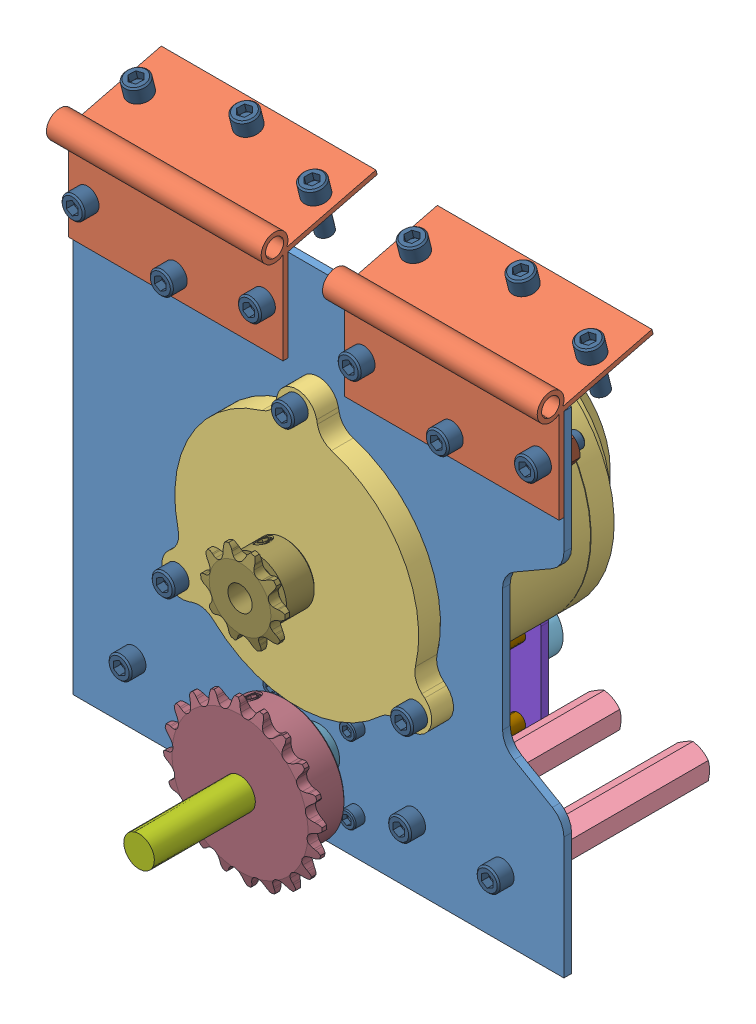
SolidWorks assembly Subassem - Steering Motor, configuration Default. Lengths in mm.
Overall size (203.2 231.02 172.82).
54 component instances, 14 part files, 101 mates.
Components (placement in the parent):
- Motor Mount-1: Motor Mount [Default] at origin size (203.2 203.2 3.17)
- Hinges-1: Hinges [Default] at (0 105.8998 5.5035) size (203.2 49.24 48.03)
- Motor-1: Motor [Default] at (0 0 -78.6404) x (1 0 0) z (0 -1 0) size (111.79 120.23 113.74)
- Standoff 3in 0.25-20-1: Standoff 3in 0.25-20 [92230A345] at (76.2 -76.2 -41.275) size (12.7 14.66 77.95)
- Standoff 3in 0.25-20-2: Standoff 3in 0.25-20 [92230A345] at (39.5531 -76.2 -41.275) size (12.7 14.66 77.95)
- Standoff 3in 0.25-20-3: Standoff 3in 0.25-20 [92230A345] at (-39.5531 -76.2 -41.275) size (12.7 14.66 77.95)
- Standoff 3in 0.25-20-4: Standoff 3in 0.25-20 [92230A345] at (-76.2 -76.2 -41.275) size (12.7 14.66 77.95)
- Potentiometer-1: Potentiometer [Default] at (0 -69.8325 -90.17) x (1 0 0) z (0 -1 0) size (22.23 39.37 22.23)
- Shaft Coupler 0.25-0.50-1: Shaft Coupler 0.25-0.50 [3084K31] at (0 -69.8325 -39.6875) x (0 0 -1) z (-0.419694 0.907666 0) size (47.67 31.75 31.75)
- Shaft 0.5in-1: Shaft 0.5in [Default] at (0 -69.85 17.145) x (-0.735553 0.677467 0) z (0 0 1) size (12.7 12.7 114.3)
- Pot Plate-2: Pot Plate [Default] at (0 -69.8325 -68.2625) size (50.8 50.8 3.17)
- Standoff 3in 8-32-1: Standoff 3in 8-32 [Default] at (-15.875 -53.9575 -34.925) size (6.35 6.35 63.5)
- Standoff 3in 8-32-7: Standoff 3in 8-32 [Default] at (15.875 -85.7075 -34.925) size (6.35 6.35 63.5)
- Standoff 3in 8-32-8: Standoff 3in 8-32 [Default] at (15.875 -53.9575 -34.925) size (6.35 6.35 63.5)
- Standoff 3in 8-32-9: Standoff 3in 8-32 [Default] at (-15.875 -85.7425 -34.925) size (6.35 6.35 63.5)
- Socket Head Cap Screw_AI-1: Socket Head Cap Screw_AI [HX-SHCS 0.25-28x0.625x0.625-N] at (-76.2 -76.2 6.35) x (0 0 -1) z (1 0 0) size (22.23 9.53 9.53)
- Socket Head Cap Screw_AI-2: Socket Head Cap Screw_AI [HX-SHCS 0.25-28x0.625x0.625-N] at (-39.5531 -76.2 6.35) x (0 0 -1) z (1 0 0) size (22.23 9.53 9.53)
- Socket Head Cap Screw_AI-3: Socket Head Cap Screw_AI [HX-SHCS 0.25-28x0.625x0.625-N] at (39.5531 -76.2 6.35) x (0 0 -1) z (1 0 0) size (22.23 9.53 9.53)
- Socket Head Cap Screw_AI-4: Socket Head Cap Screw_AI [HX-SHCS 0.25-28x0.625x0.625-N] at (76.2 -76.2 6.35) x (0 0 -1) z (1 0 0) size (22.23 9.53 9.53)
- Socket Head Cap Screw_AI-6: Socket Head Cap Screw_AI [HX-SHCS 0.25-28x0.625x0.625-N] at (-93.6625 80.9625 8.3344) x (0 0 -1) z (1 0 0) size (22.23 9.53 9.53)
- Socket Head Cap Screw_AI-7: Socket Head Cap Screw_AI [HX-SHCS 0.25-28x0.625x0.625-N] at (-57.15 72.2313 8.3344) x (0 0 -1) z (1 0 0) size (22.23 9.53 9.53)
- Socket Head Cap Screw_AI-8: Socket Head Cap Screw_AI [HX-SHCS 0.25-28x0.625x0.625-N] at (-20.6375 80.9625 8.3344) x (0 0 -1) z (1 0 0) size (22.23 9.53 9.53)
- Socket Head Cap Screw_AI-9: Socket Head Cap Screw_AI [HX-SHCS 0.25-28x0.625x0.625-N] at (20.6375 80.9625 8.3344) x (0 0 -1) z (1 0 0) size (22.23 9.53 9.53)
- Socket Head Cap Screw_AI-10: Socket Head Cap Screw_AI [HX-SHCS 0.25-28x0.625x0.625-N] at (57.15 72.2313 8.3344) x (0 0 -1) z (1 0 0) size (22.23 9.53 9.53)
- Socket Head Cap Screw_AI-11: Socket Head Cap Screw_AI [HX-SHCS 0.25-28x0.625x0.625-N] at (93.6625 80.9625 8.3344) x (0 0 -1) z (1 0 0) size (22.23 9.53 9.53)
- Socket Head Cap Screw_AI-31: Socket Head Cap Screw_AI [HX-SHCS 0.25-20x1x1-N] at (0 57 15.35) x (0 0 -1) z (1 0 0) size (31.75 9.53 9.53)
- Socket Head Cap Screw_AI-32: Socket Head Cap Screw_AI [HX-SHCS 0.25-20x1x1-N] at (-49.3634 -28.5 15.35) x (0 0 -1) z (1 0 0) size (31.75 9.53 9.53)
- Socket Head Cap Screw_AI-33: Socket Head Cap Screw_AI [HX-SHCS 0.25-20x1x1-N] at (49.3634 -28.5 15.35) x (0 0 -1) z (1 0 0) size (31.75 9.53 9.53)
- Hex Nut_AI-2: Hex Nut_AI [HNUT 0.2500-28-D-N] at (-93.6625 80.9625 -3.175) size (11.11 12.83 5.74)
- Hex Nut_AI-3: Hex Nut_AI [HNUT 0.2500-28-D-N] at (-57.15 72.2313 -4.085) size (11.11 12.83 5.74)
- Hex Nut_AI-4: Hex Nut_AI [HNUT 0.2500-28-D-N] at (-20.6375 80.9625 -8.9154) x (0.923728 0.383049 0) z (0 0 -1) size (11.11 12.83 5.74)
- Hex Nut_AI-5: Hex Nut_AI [HNUT 0.2500-28-D-N] at (20.6375 80.9625 -8.9154) x (0.923728 0.383049 0) z (0 0 -1) size (11.11 12.83 5.74)
- Hex Nut_AI-6: Hex Nut_AI [HNUT 0.2500-28-D-N] at (57.15 72.2313 -8.9154) x (0.923728 0.383049 0) z (0 0 -1) size (11.11 12.83 5.74)
- Hex Nut_AI-7: Hex Nut_AI [HNUT 0.2500-28-D-N] at (93.6625 80.9625 -8.9154) x (0.923728 0.383049 0) z (0 0 -1) size (11.11 12.83 5.74)
- Hex Nut_AI-8: Hex Nut_AI [HNUT 0.2500-20-D-N] at (0 57 -8.9154) x (0.923728 0.383049 0) z (0 0 -1) size (11.11 12.83 5.74)
- Hex Nut_AI-9: Hex Nut_AI [HNUT 0.2500-20-D-N] at (-49.3634 -28.5 -8.9154) x (0.923728 0.383049 0) z (0 0 -1) size (11.11 12.83 5.74)
- Hex Nut_AI-10: Hex Nut_AI [HNUT 0.2500-20-D-N] at (49.3634 -28.5 -8.9154) x (0.923728 0.383049 0) z (0 0 -1) size (11.11 12.83 5.74)
- Socket Head Cap Screw_AI-35: Socket Head Cap Screw_AI [HX-SHCS 0.164-32x0.5x0.5-N] at (-15.875 -53.9575 4.1656) x (0 0 -1) z (1 0 0) size (16.87 6.86 6.86)
- Socket Head Cap Screw_AI-36: Socket Head Cap Screw_AI [HX-SHCS 0.164-32x0.5x0.5-N] at (-15.875 -85.7425 4.1656) x (0 0 -1) z (1 0 0) size (16.87 6.86 6.86)
- Socket Head Cap Screw_AI-37: Socket Head Cap Screw_AI [HX-SHCS 0.164-32x0.5x0.5-N] at (15.875 -53.9575 4.1656) x (0 0 -1) z (1 0 0) size (16.87 6.86 6.86)
- Socket Head Cap Screw_AI-38: Socket Head Cap Screw_AI [HX-SHCS 0.164-32x0.5x0.5-N] at (15.875 -85.7425 4.1656) x (0 0 -1) z (1 0 0) size (16.87 6.86 6.86)
- Socket Head Cap Screw_AI-39: Socket Head Cap Screw_AI [HX-SHCS 0.164-32x0.5x0.5-N] at (15.875 -53.9575 -74.0156) x (0 0 1) z (-1 0 0) size (16.87 6.86 6.86)
- Socket Head Cap Screw_AI-40: Socket Head Cap Screw_AI [HX-SHCS 0.164-32x0.5x0.5-N] at (15.875 -85.7075 -74.0156) x (0 0 1) z (-1 0 0) size (16.87 6.86 6.86)
- Socket Head Cap Screw_AI-41: Socket Head Cap Screw_AI [HX-SHCS 0.164-32x0.5x0.5-N] at (-15.875 -85.7075 -74.0156) x (0 0 1) z (-1 0 0) size (16.87 6.86 6.86)
- Socket Head Cap Screw_AI-42: Socket Head Cap Screw_AI [HX-SHCS 0.164-32x0.5x0.5-N] at (-15.875 -53.9575 -74.0156) x (0 0 1) z (-1 0 0) size (16.87 6.86 6.86)
- Socket Head Cap Screw_AI-44: Socket Head Cap Screw_AI [HX-SHCS 0.25-28x0.625x0.625-N] at (-93.6625 114.6795 -18.0082) x (0 -0.970296 -0.241922) z (0.241922 -0.234736 0.941474) size (22.23 9.53 9.53)
- Socket Head Cap Screw_AI-45: Socket Head Cap Screw_AI [HX-SHCS 0.25-28x0.625x0.625-N] at (-57.15 116.7918 -26.4801) x (0 -0.970296 -0.241922) z (0.241922 -0.234736 0.941474) size (22.23 9.53 9.53)
- Socket Head Cap Screw_AI-46: Socket Head Cap Screw_AI [HX-SHCS 0.25-28x0.625x0.625-N] at (-20.6375 114.6795 -18.0082) x (0 -0.970296 -0.241922) z (0.241922 -0.234736 0.941474) size (22.23 9.53 9.53)
- Socket Head Cap Screw_AI-47: Socket Head Cap Screw_AI [HX-SHCS 0.25-28x0.625x0.625-N] at (20.6375 114.6795 -18.0082) x (0 -0.970296 -0.241922) z (0.241922 -0.234736 0.941474) size (22.23 9.53 9.53)
- Socket Head Cap Screw_AI-48: Socket Head Cap Screw_AI [HX-SHCS 0.25-28x0.625x0.625-N] at (57.15 116.7918 -26.4801) x (0 -0.970296 -0.241922) z (0.241922 -0.234736 0.941474) size (22.23 9.53 9.53)
- Socket Head Cap Screw_AI-49: Socket Head Cap Screw_AI [HX-SHCS 0.25-28x0.625x0.625-N] at (93.6625 114.6795 -18.0082) x (0 -0.970296 -0.241922) z (0.241922 -0.234736 0.941474) size (22.23 9.53 9.53)
- Sprocket - 10 Tooth-1: Sprocket - 10 Tooth [6280K321] at (0 0 30.3614) x (-0.923728 -0.383049 0) z (0 0 -1) size (33.82 35.03 19.05)
- Sprocket - 15 Tooth-1: Sprocket - 15 Tooth [6280K384] at (0 -69.85 30.3614) x (-0.923728 -0.383049 0) z (0 0 -1) size (65.79 65.79 19.05)
- Roller Bearing 0.5in-1: Roller Bearing 0.5in [5905K23] at (0 -69.85 -2.3118) x (0.999532 0.030579 0) z (0 0 1) size (17.46 17.46 12.7)
Mates (geometry in assembly coordinates):
- Concentric1: concentric aligned: cylinder of Motor Mount-1 through (-93.6625 80.9625 0) axis (0 0 1) radius 3.2639; cylinder of Hinges-1 through (-93.6625 80.9625 0) axis (0 0 1) radius 4.3656
- Concentric2: concentric aligned: cylinder of Motor Mount-1 through (-57.15 72.2313 0) axis (0 0 1) radius 3.2639; cylinder of Hinges-1 through (-57.15 72.2313 0) axis (0 0 1) radius 4.3656
- Coincident1: coincident anti-aligned: plane of Motor Mount-1 through (0 0 0) normal (0 0 1); plane of Hinges-1 through (101.6 105.8998 0) normal (0 0 -1)
- Coincident2: coincident aligned: circle of Motor Mount-1; circle of Motor-1
- Concentric3: concentric anti-aligned: cylinder of Motor Mount-1 through (-49.3634 -28.5 -3.175) axis (0 0 1) radius 4.25; cylinder of Motor-1 through (-49.3634 -28.5 9) axis (0 0 -1) radius 4.25
- Concentric7: concentric anti-aligned: circle of Motor Mount-1; circle of Standoff 3in 0.25-20-1
- Coincident5: coincident anti-aligned: plane of Motor Mount-1 through (0 0 -3.175) normal (0 0 -1); plane of Standoff 3in 0.25-20-1 through (76.2 -68.8677 -3.175) normal (0 0 1)
- Coincident6: coincident anti-aligned: plane of Motor Mount-1 through (0 0 -3.175) normal (0 0 -1); plane of Standoff 3in 0.25-20-2 through (39.5531 -68.8677 -3.175) normal (0 0 1)
- Concentric8: concentric anti-aligned: circle of Motor Mount-1; circle of Standoff 3in 0.25-20-2
- Concentric9: concentric anti-aligned: circle of Motor Mount-1; circle of Standoff 3in 0.25-20-3
- Coincident7: coincident anti-aligned: plane of Motor Mount-1 through (0 0 -3.175) normal (0 0 -1); plane of Standoff 3in 0.25-20-3 through (-39.5531 -68.8677 -3.175) normal (0 0 1)
- Concentric10: concentric anti-aligned: circle of Motor Mount-1; circle of Standoff 3in 0.25-20-4
- Coincident8: coincident anti-aligned: plane of Motor Mount-1 through (0 0 -3.175) normal (0 0 -1); plane of Standoff 3in 0.25-20-4 through (-76.2 -68.8677 -3.175) normal (0 0 1)
- Concentric13: concentric aligned: cylinder of Motor Mount-1 through (-76.2 -76.2 0) axis (0 0 1) radius 3.2639; cylinder of Socket Head Cap Screw_AI-1 through (-76.2 -76.2 38.1) axis (0 0 1) radius 4.7625
- Coincident11: coincident anti-aligned: plane of Motor Mount-1 through (0 0 0) normal (0 0 1); plane of Socket Head Cap Screw_AI-1 through (-76.2 -71.4375 0) normal (0 0 -1)
- Concentric14: concentric aligned: cylinder of Motor Mount-1 through (-39.5531 -76.2 0) axis (0 0 1) radius 3.2639; cylinder of Socket Head Cap Screw_AI-2 through (-39.5531 -76.2 38.1) axis (0 0 1) radius 4.7625
- Coincident12: coincident anti-aligned: plane of Motor Mount-1 through (0 0 0) normal (0 0 1); plane of Socket Head Cap Screw_AI-2 through (-39.5531 -71.4375 0) normal (0 0 -1)
- Concentric15: concentric aligned: cylinder of Motor Mount-1 through (39.5531 -76.2 0) axis (0 0 1) radius 3.2639; cylinder of Socket Head Cap Screw_AI-3 through (39.5531 -76.2 38.1) axis (0 0 1) radius 4.7625
- Coincident13: coincident anti-aligned: plane of Motor Mount-1 through (0 0 0) normal (0 0 1); plane of Socket Head Cap Screw_AI-3 through (39.5531 -71.4375 0) normal (0 0 -1)
- Concentric16: concentric aligned: cylinder of Motor Mount-1 through (76.2 -76.2 0) axis (0 0 1) radius 3.2639; cylinder of Socket Head Cap Screw_AI-4 through (76.2 -76.2 38.1) axis (0 0 1) radius 4.7625
- Coincident14: coincident anti-aligned: plane of Motor Mount-1 through (0 0 0) normal (0 0 1); plane of Socket Head Cap Screw_AI-4 through (76.2 -71.4375 0) normal (0 0 -1)
- Concentric18: concentric aligned: cylinder of Hinges-1 through (-93.6625 80.9625 0) axis (0 0 1) radius 4.3656; cylinder of Socket Head Cap Screw_AI-6 through (-93.6625 80.9625 40.0844) axis (0 0 1) radius 4.7625
- Coincident16: coincident anti-aligned: plane of Hinges-1 through (101.6 105.8998 1.9844) normal (0 0 1); plane of Socket Head Cap Screw_AI-6 through (-93.6625 85.725 1.9844) normal (0 0 -1)
- Concentric19: concentric aligned: cylinder of Hinges-1 through (-57.15 72.2313 0) axis (0 0 1) radius 4.3656; cylinder of Socket Head Cap Screw_AI-7 through (-57.15 72.2313 40.0844) axis (0 0 1) radius 4.7625
- Coincident17: coincident anti-aligned: plane of Hinges-1 through (101.6 105.8998 1.9844) normal (0 0 1); plane of Socket Head Cap Screw_AI-7 through (-57.15 76.9938 1.9844) normal (0 0 -1)
- Concentric20: concentric aligned: cylinder of Hinges-1 through (-20.6375 80.9625 0) axis (0 0 1) radius 4.3656; cylinder of Socket Head Cap Screw_AI-8 through (-20.6375 80.9625 40.0844) axis (0 0 1) radius 4.7625
- Coincident18: coincident anti-aligned: plane of Hinges-1 through (101.6 105.8998 1.9844) normal (0 0 1); plane of Socket Head Cap Screw_AI-8 through (-20.6375 85.725 1.9844) normal (0 0 -1)
- Concentric21: concentric aligned: cylinder of Hinges-1 through (20.6375 80.9625 0) axis (0 0 1) radius 4.3656; cylinder of Socket Head Cap Screw_AI-9 through (20.6375 80.9625 40.0844) axis (0 0 1) radius 4.7625
- Coincident19: coincident anti-aligned: plane of Hinges-1 through (101.6 105.8998 1.9844) normal (0 0 1); plane of Socket Head Cap Screw_AI-9 through (20.6375 85.725 1.9844) normal (0 0 -1)
- Concentric22: concentric aligned: cylinder of Hinges-1 through (57.15 72.2313 0) axis (0 0 1) radius 4.3656; cylinder of Socket Head Cap Screw_AI-10 through (57.15 72.2313 40.0844) axis (0 0 1) radius 4.7625
- Coincident20: coincident anti-aligned: plane of Hinges-1 through (101.6 105.8998 1.9844) normal (0 0 1); plane of Socket Head Cap Screw_AI-10 through (57.15 76.9938 1.9844) normal (0 0 -1)
- Concentric23: concentric aligned: cylinder of Hinges-1 through (93.6625 80.9625 0) axis (0 0 1) radius 4.3656; cylinder of Socket Head Cap Screw_AI-11 through (93.6625 80.9625 40.0844) axis (0 0 1) radius 4.7625
- Coincident21: coincident anti-aligned: plane of Hinges-1 through (101.6 105.8998 1.9844) normal (0 0 1); plane of Socket Head Cap Screw_AI-11 through (93.6625 85.725 1.9844) normal (0 0 -1)
- Concentric32: concentric anti-aligned: cylinder of Potentiometer-1 through (0 -69.8325 -90.17) axis (0 0 -1) radius 3.175; cylinder of Shaft Coupler 0.25-0.50-1 through (0 -69.8325 -15.875) axis (0 0 1) radius 2.9845
- Coincident31: coincident anti-aligned: plane of Potentiometer-1 through (5.5562 -69.8325 -63.5) normal (0 0 1); plane of Shaft Coupler 0.25-0.50-1 through (4.897 -80.4233 -63.5) normal (0 0 -1)
- Coincident36: coincident anti-aligned: plane of Shaft Coupler 0.25-0.50-1 through (7.7465 -48.7607 -40.005) normal (0 0 1); plane of Shaft 0.5in-1 through (0 -69.85 -40.005) normal (0 0 -1)
- Concentric46: concentric anti-aligned: cylinder of Motor-1 through (0 57 9) axis (0 0 -1) radius 4.25; cylinder of Socket Head Cap Screw_AI-31 through (0 57 47.1) axis (0 0 1) radius 4.7625
- Coincident45: coincident anti-aligned: plane of Motor-1 through (0 54.8512 9) normal (0 0 1); plane of Socket Head Cap Screw_AI-31 through (0 61.7625 9) normal (0 0 -1)
- Concentric47: concentric anti-aligned: cylinder of Motor-1 through (-49.3634 -28.5 9) axis (0 0 -1) radius 4.25; cylinder of Socket Head Cap Screw_AI-32 through (-49.3634 -28.5 47.1) axis (0 0 1) radius 4.7625
- Coincident46: coincident anti-aligned: plane of Motor-1 through (0 54.8512 9) normal (0 0 1); plane of Socket Head Cap Screw_AI-32 through (-49.3634 -23.7375 9) normal (0 0 -1)
- Concentric48: concentric anti-aligned: cylinder of Motor-1 through (49.3634 -28.5 9) axis (0 0 -1) radius 4.25; cylinder of Socket Head Cap Screw_AI-33 through (49.3634 -28.5 47.1) axis (0 0 1) radius 4.7625
- Coincident47: coincident anti-aligned: plane of Motor-1 through (0 54.8512 9) normal (0 0 1); plane of Socket Head Cap Screw_AI-33 through (49.3634 -23.7375 9) normal (0 0 -1)
- Concentric51: concentric aligned: cylinder of Socket Head Cap Screw_AI-6 through (-93.6625 80.9625 40.0844) axis (0 0 1) radius 3.175; cylinder of Hex Nut_AI-2 through (-93.6625 80.9625 -28.2125) axis (0 0 1) radius 3.175
- Concentric52: concentric aligned: cylinder of Socket Head Cap Screw_AI-7 through (-57.15 72.2313 40.0844) axis (0 0 1) radius 3.175; cylinder of Hex Nut_AI-3 through (-57.15 72.2313 -29.1225) axis (0 0 1) radius 3.175
- Concentric53: concentric anti-aligned: cylinder of Motor Mount-1 through (-20.6375 80.9625 0) axis (0 0 1) radius 3.2639; cylinder of Hex Nut_AI-4 through (-20.6375 80.9625 16.1221) axis (0 0 -1) radius 3.175
- Coincident50: coincident anti-aligned: plane of Motor Mount-1 through (0 0 -3.175) normal (0 0 -1); plane of Hex Nut_AI-4 through (-18.1799 75.036 -3.175) normal (0 0 1)
- Concentric54: concentric anti-aligned: cylinder of Motor Mount-1 through (20.6375 80.9625 0) axis (0 0 1) radius 3.2639; cylinder of Hex Nut_AI-5 through (20.6375 80.9625 16.1221) axis (0 0 -1) radius 3.175
- Coincident51: coincident anti-aligned: plane of Motor Mount-1 through (0 0 -3.175) normal (0 0 -1); plane of Hex Nut_AI-5 through (23.0951 75.036 -3.175) normal (0 0 1)
- Concentric55: concentric anti-aligned: cylinder of Motor Mount-1 through (57.15 72.2313 0) axis (0 0 1) radius 3.2639; cylinder of Hex Nut_AI-6 through (57.15 72.2313 16.1221) axis (0 0 -1) radius 3.175
- Coincident52: coincident anti-aligned: plane of Motor Mount-1 through (0 0 -3.175) normal (0 0 -1); plane of Hex Nut_AI-6 through (59.6076 66.3048 -3.175) normal (0 0 1)
- Concentric56: concentric anti-aligned: cylinder of Motor Mount-1 through (93.6625 80.9625 0) axis (0 0 1) radius 3.2639; cylinder of Hex Nut_AI-7 through (93.6625 80.9625 16.1221) axis (0 0 -1) radius 3.175
- Coincident53: coincident anti-aligned: plane of Motor Mount-1 through (0 0 -3.175) normal (0 0 -1); plane of Hex Nut_AI-7 through (96.1201 75.036 -3.175) normal (0 0 1)
- Concentric57: concentric anti-aligned: cylinder of Motor Mount-1 through (0 57 -3.175) axis (0 0 1) radius 4.25; cylinder of Hex Nut_AI-8 through (0 57 16.1221) axis (0 0 -1) radius 3.175
- Coincident54: coincident anti-aligned: plane of Motor Mount-1 through (0 0 -3.175) normal (0 0 -1); plane of Hex Nut_AI-8 through (2.4576 51.0735 -3.175) normal (0 0 1)
- Concentric58: concentric anti-aligned: cylinder of Motor Mount-1 through (-49.3634 -28.5 -3.175) axis (0 0 1) radius 4.25; cylinder of Hex Nut_AI-9 through (-49.3634 -28.5 16.1221) axis (0 0 -1) radius 3.175
- Coincident55: coincident anti-aligned: plane of Motor Mount-1 through (0 0 -3.175) normal (0 0 -1); plane of Hex Nut_AI-9 through (-46.9059 -34.4265 -3.175) normal (0 0 1)
- Concentric59: concentric anti-aligned: cylinder of Motor Mount-1 through (49.3634 -28.5 -3.175) axis (0 0 1) radius 4.25; cylinder of Hex Nut_AI-10 through (49.3634 -28.5 16.1221) axis (0 0 -1) radius 3.175
- Coincident56: coincident anti-aligned: plane of Motor Mount-1 through (0 0 -3.175) normal (0 0 -1); plane of Hex Nut_AI-10 through (51.821 -34.4265 -3.175) normal (0 0 1)
- Coincident57: coincident anti-aligned: plane of Motor Mount-1 through (0 0 -3.175) normal (0 0 -1); plane of Hex Nut_AI-2 through (-93.6625 87.3783 -3.175) normal (0 0 1)
- Coincident60: coincident aligned: circle of Motor Mount-1; circle of Standoff 3in 8-32-9
- Coincident61: coincident aligned: circle of Motor Mount-1; circle of Standoff 3in 8-32-8
- Coincident63: coincident aligned: circle of Pot Plate-2; circle of Standoff 3in 8-32-1
- Coincident64: coincident aligned: circle of Pot Plate-2; circle of Standoff 3in 8-32-7
- Coincident65: coincident anti-aligned: circle of Potentiometer-1; circle of Pot Plate-2
- Concentric63: concentric aligned: cylinder of Motor Mount-1 through (-15.875 -53.9575 0) axis (0 0 1) radius 2.1526; cylinder of Socket Head Cap Screw_AI-35 through (-15.875 -53.9575 35.9156) axis (0 0 1) radius 3.429
- Coincident67: coincident anti-aligned: plane of Motor Mount-1 through (0 0 0) normal (0 0 1); plane of Socket Head Cap Screw_AI-35 through (-15.875 -50.5285 0) normal (0 0 -1)
- Concentric64: concentric aligned: cylinder of Motor Mount-1 through (-15.875 -85.7425 0) axis (0 0 1) radius 2.1526; cylinder of Socket Head Cap Screw_AI-36 through (-15.875 -85.7425 35.9156) axis (0 0 1) radius 3.429
- Coincident68: coincident anti-aligned: plane of Motor Mount-1 through (0 0 0) normal (0 0 1); plane of Socket Head Cap Screw_AI-36 through (-15.875 -82.3135 0) normal (0 0 -1)
- Concentric65: concentric aligned: cylinder of Motor Mount-1 through (15.875 -53.9575 0) axis (0 0 1) radius 2.1526; cylinder of Socket Head Cap Screw_AI-37 through (15.875 -53.9575 35.9156) axis (0 0 1) radius 3.429
- Coincident69: coincident anti-aligned: plane of Motor Mount-1 through (0 0 0) normal (0 0 1); plane of Socket Head Cap Screw_AI-37 through (15.875 -50.5285 0) normal (0 0 -1)
- Concentric66: concentric aligned: cylinder of Motor Mount-1 through (15.875 -85.7425 0) axis (0 0 1) radius 2.1526; cylinder of Socket Head Cap Screw_AI-38 through (15.875 -85.7425 35.9156) axis (0 0 1) radius 3.429
- Coincident70: coincident anti-aligned: plane of Motor Mount-1 through (0 0 0) normal (0 0 1); plane of Socket Head Cap Screw_AI-38 through (15.875 -82.3135 0) normal (0 0 -1)
- Concentric67: concentric anti-aligned: cylinder of Pot Plate-2 through (15.875 -53.9575 -66.675) axis (0 0 1) radius 2.1526; cylinder of Socket Head Cap Screw_AI-39 through (15.875 -53.9575 -105.7656) axis (0 0 -1) radius 3.429
- Coincident71: coincident anti-aligned: plane of Pot Plate-2 through (0 -69.8325 -69.85) normal (0 0 -1); plane of Socket Head Cap Screw_AI-39 through (15.875 -50.5285 -69.85) normal (0 0 1)
- Concentric68: concentric anti-aligned: cylinder of Pot Plate-2 through (15.875 -85.7075 -66.675) axis (0 0 1) radius 2.1526; cylinder of Socket Head Cap Screw_AI-40 through (15.875 -85.7075 -105.7656) axis (0 0 -1) radius 3.429
- Coincident72: coincident anti-aligned: plane of Pot Plate-2 through (0 -69.8325 -69.85) normal (0 0 -1); plane of Socket Head Cap Screw_AI-40 through (15.875 -82.2785 -69.85) normal (0 0 1)
- Concentric69: concentric anti-aligned: cylinder of Pot Plate-2 through (-15.875 -85.7075 -66.675) axis (0 0 1) radius 2.1526; cylinder of Socket Head Cap Screw_AI-41 through (-15.875 -85.7075 -105.7656) axis (0 0 -1) radius 3.429
- Coincident73: coincident anti-aligned: plane of Pot Plate-2 through (0 -69.8325 -69.85) normal (0 0 -1); plane of Socket Head Cap Screw_AI-41 through (-15.875 -82.2785 -69.85) normal (0 0 1)
- Concentric70: concentric anti-aligned: cylinder of Pot Plate-2 through (-15.875 -53.9575 -66.675) axis (0 0 1) radius 2.1526; cylinder of Socket Head Cap Screw_AI-42 through (-15.875 -53.9575 -105.7656) axis (0 0 -1) radius 3.429
- Coincident74: coincident anti-aligned: plane of Pot Plate-2 through (0 -69.8325 -69.85) normal (0 0 -1); plane of Socket Head Cap Screw_AI-42 through (-15.875 -50.5285 -69.85) normal (0 0 1)
- Concentric72: concentric aligned: cylinder of Hinges-1 through (-93.6625 106.5927 -20.0245) axis (0 0.970296 0.241922) radius 4.3656; cylinder of Socket Head Cap Screw_AI-44 through (-93.6625 145.4864 -10.3272) axis (0 0.970296 0.241922) radius 4.7625
- Coincident76: coincident anti-aligned: plane of Hinges-1 through (101.6 102.4852 4.6521) normal (0 0.970296 0.241922); plane of Socket Head Cap Screw_AI-44 through (-89.0415 108.7968 -20.6623) normal (0 -0.970296 -0.241922)
- Concentric73: concentric aligned: cylinder of Hinges-1 through (-57.15 108.7049 -28.4964) axis (0 0.970296 0.241922) radius 4.3656; cylinder of Socket Head Cap Screw_AI-45 through (-57.15 147.5986 -18.7991) axis (0 0.970296 0.241922) radius 4.7625
- Coincident77: coincident anti-aligned: plane of Hinges-1 through (101.6 102.4852 4.6521) normal (0 0.970296 0.241922); plane of Socket Head Cap Screw_AI-45 through (-52.529 110.9091 -29.1342) normal (0 -0.970296 -0.241922)
- Concentric74: concentric aligned: cylinder of Hinges-1 through (-20.6375 106.5927 -20.0245) axis (0 0.970296 0.241922) radius 4.3656; cylinder of Socket Head Cap Screw_AI-46 through (-20.6375 145.4864 -10.3272) axis (0 0.970296 0.241922) radius 4.7625
- Coincident78: coincident anti-aligned: plane of Hinges-1 through (101.6 102.4852 4.6521) normal (0 0.970296 0.241922); plane of Socket Head Cap Screw_AI-46 through (-16.0165 108.7968 -20.6623) normal (0 -0.970296 -0.241922)
- Concentric75: concentric aligned: cylinder of Hinges-1 through (20.6375 106.5927 -20.0245) axis (0 0.970296 0.241922) radius 4.3656; cylinder of Socket Head Cap Screw_AI-47 through (20.6375 145.4864 -10.3272) axis (0 0.970296 0.241922) radius 4.7625
- Coincident79: coincident anti-aligned: plane of Hinges-1 through (101.6 102.4852 4.6521) normal (0 0.970296 0.241922); plane of Socket Head Cap Screw_AI-47 through (25.2585 108.7968 -20.6623) normal (0 -0.970296 -0.241922)
- Concentric76: concentric aligned: cylinder of Hinges-1 through (57.15 108.7049 -28.4964) axis (0 0.970296 0.241922) radius 4.3656; cylinder of Socket Head Cap Screw_AI-48 through (57.15 147.5986 -18.7991) axis (0 0.970296 0.241922) radius 4.7625
- Coincident80: coincident anti-aligned: plane of Hinges-1 through (101.6 102.4852 4.6521) normal (0 0.970296 0.241922); plane of Socket Head Cap Screw_AI-48 through (61.771 110.9091 -29.1342) normal (0 -0.970296 -0.241922)
- Concentric77: concentric aligned: cylinder of Hinges-1 through (93.6625 106.5927 -20.0245) axis (0 0.970296 0.241922) radius 4.3656; cylinder of Socket Head Cap Screw_AI-49 through (93.6625 145.4864 -10.3272) axis (0 0.970296 0.241922) radius 4.7625
- Coincident81: coincident anti-aligned: plane of Hinges-1 through (101.6 102.4852 4.6521) normal (0 0.970296 0.241922); plane of Socket Head Cap Screw_AI-49 through (98.2835 108.7968 -20.6623) normal (0 -0.970296 -0.241922)
- Concentric78: concentric anti-aligned: cylinder of Motor-1 through (0 0 21.7) axis (0 0 -1) radius 5; cylinder of Sprocket - 10 Tooth-1 through (0 0 13.445) axis (0 0 1) radius 5.0165
- Distance1: distance = 4.445 mm anti-aligned: plane of Motor-1 through (0 54.8512 9) normal (0 0 1); plane of Sprocket - 10 Tooth-1 through (0 0 13.445) normal (0 0 -1)
- Concentric79: concentric anti-aligned: cylinder of Shaft 0.5in-1 through (0 -69.85 74.295) axis (0 0 -1) radius 6.35; cylinder of Sprocket - 15 Tooth-1 through (0 -69.85 13.445) axis (0 0 1) radius 6.35
- Coincident82: coincident aligned: plane of Sprocket - 10 Tooth-1 through (4.8848 -11.7798 32.495) normal (0 0 1); plane of Sprocket - 15 Tooth-1 through (10.7883 -95.8661 32.495) normal (0 0 1)
- Concentric80: concentric aligned: cylinder of Motor Mount-1 through (0 -69.85 -3.175) axis (0 0 1) radius 8.7312; cylinder of Roller Bearing 0.5in-1 through (0 -69.85 4.0382) axis (0 0 1) radius 8.7312
- Concentric81: concentric anti-aligned: cylinder of Motor Mount-1 through (0 -69.85 -3.175) axis (0 0 1) radius 8.7312; cylinder of Shaft 0.5in-1 through (0 -69.85 74.295) axis (0 0 -1) radius 6.35
- Concentric83: concentric anti-aligned: cylinder of Pot Plate-2 through (15.875 -53.9575 -66.675) axis (0 0 1) radius 2.1526; cylinder of Standoff 3in 8-32-8 through (15.875 -53.9575 -3.175) axis (0 0 -1) radius 2.1526
- Concentric86: concentric anti-aligned: cylinder of Motor Mount-1 through (-15.875 -53.9575 0) axis (0 0 1) radius 2.1526; cylinder of Standoff 3in 8-32-1 through (-15.875 -53.9575 -3.175) axis (0 0 -1) radius 3.175
- Coincident83: coincident anti-aligned: plane of Pot Plate-2 through (0 -69.8325 -66.675) normal (0 0 1); plane of Standoff 3in 8-32-9 through (-15.875 -85.7425 -66.675) normal (0 0 -1)
